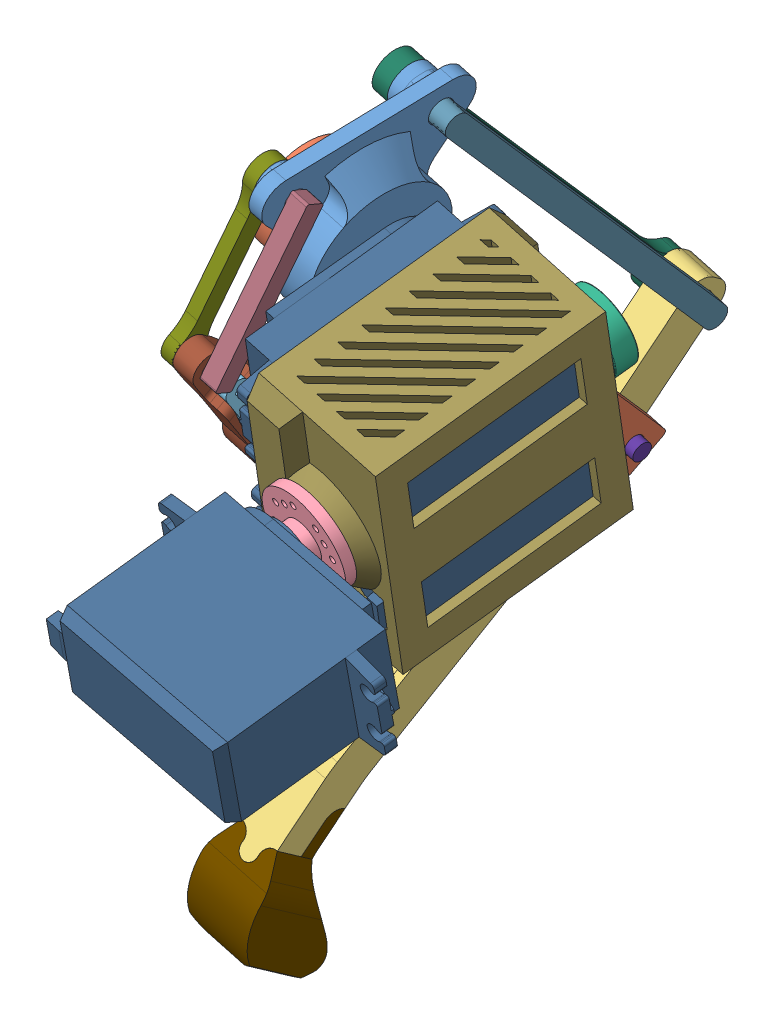
SolidWorks assembly Leg 0, configuration Default. Lengths in mm.
Overall size (103.06 201.69 173.07).
31 component instances, 18 part files, 41 mates.
Components (placement in the parent):
- RearRotatingPiece-1: RearRotatingPiece [Default] at (17.8529 197.1276 29.9823) x (-0.180704 -0.967706 0.175759) z (-0.0444 0.186545 0.981443) size (44.28 13.7 43.21)
- RearUpperLeg-1: RearUpperLeg [Default] at (9.3497 122.3315 -43.4021) x (0.169452 0.64499 -0.745167) z (0.982535 -0.169547 0.076676) size (22 116.4 18)
- RearLowerLeg-1: RearLowerLeg [Default] at (-4.4037 50.9577 33.7008) x (0.037011 0.581891 0.812424) z (-0.982535 0.169547 -0.076676) size (20.21 126 9.59)
- Circle Rudder-1: Circle Rudder [默认] at (18.0109 173.864 63.2452) x (0.470065 -0.866717 -0.166853) z (-0.874709 -0.432175 -0.219336) size (20.8 5.5 20.8)
- Double_Blade_Rudder-1: Double_Blade_Rudder [默认] at (-13.5228 170.7521 41.1436) x (-0.171815 -0.668394 0.723692) z (0.07145 0.724226 0.685851) size (12.2 5.5 38)
- 688ZZ Bearing Assembly-1: 688ZZ Bearing Assembly [Default] at (24.9725 188.558 6.5299) x (0.99278 -0.008575 0.119639) z (-0.117993 -0.24905 0.961276) size (17.99 17.98 5)
  - Outer Ring-1: Outer Ring [Default] at origin size (16 16 5)
  - Inner Ring-1: Inner Ring [Default] x (-0.241565 -0.970385 0) z (0 0 1) size (10.6 10.6 5)
  - Cage-1: Cage [Default] x (0.535517 0.844524 0) z (0 0 1) size (13.01 13.06 2.21)
  - 2mm Ball Bearing-1: 2mm Ball Bearing [Default] at (-5.0671 3.2131 0) x (0.050652 0.835774 0.546732) z (0.977207 -0.154478 0.145614) size (2 2 2)
  - 2mm Ball Bearing-2: 2mm Ball Bearing [Default] at (-5.988 -0.3789 0) x (-0.450278 0.705928 0.546732) z (0.881377 0.449412 0.145614) size (2 2 2)
  - 2mm Ball Bearing-3: 2mm Ball Bearing [Default] at (-4.6217 -3.8262 0) x (-0.779216 0.306441 0.546732) z (0.448891 0.881642 0.145614) size (2 2 2)
  - 2mm Ball Bearing-4: 2mm Ball Bearing [Default] at (-1.49 -5.812 0) x (-0.810521 -0.210096 0.546732) z (-0.155056 0.977115 0.145614) size (2 2 2)
  - 2mm Ball Bearing-5: 2mm Ball Bearing [Default] at (2.2108 -5.5778 0) x (-0.532234 -0.646383 0.546732) z (-0.699777 0.699363 0.145614) size (2 2 2)
  - 2mm Ball Bearing-6: 2mm Ball Bearing [Default] at (5.0671 -3.2131 0) x (-0.050652 -0.835774 0.546732) z (-0.977207 0.154478 0.145614) size (2 2 2)
  - 2mm Ball Bearing-7: 2mm Ball Bearing [Default] at (5.988 0.3789 0) x (0.450278 -0.705928 0.546732) z (-0.881377 -0.449412 0.145614) size (2 2 2)
  - 2mm Ball Bearing-8: 2mm Ball Bearing [Default] at (4.6217 3.8262 0) x (0.779216 -0.306441 0.546732) z (-0.448891 -0.881642 0.145614) size (2 2 2)
  - 2mm Ball Bearing-9: 2mm Ball Bearing [Default] at (1.49 5.812 0) x (0.810521 0.210096 0.546732) z (0.155056 -0.977115 0.145614) size (2 2 2)
  - 2mm Ball Bearing-10: 2mm Ball Bearing [Default] at (-2.2108 5.5778 0) x (0.532234 0.646383 0.546732) z (0.699777 -0.699363 0.145614) size (2 2 2)
- MG996R-3: MG996R [Default] at (23.0553 161.1843 107.4441) x (0.987665 -0.129781 0.087608) z (0.102937 0.959756 0.261291) size (54.5 42.75 20)
- Circle Rudder-2: Circle Rudder [默认] at (-7.0053 201.4171 28.0424) x (-0.185428 -0.85768 0.479585) z (0.015549 0.485427 0.874139) size (20.8 5.5 20.8)
- MG996R-4: MG996R [Default] at (32.1612 165.5985 34.4929) x (0.117993 0.24905 -0.961276) z (0.143886 0.953534 0.264706) size (54.5 42.75 20)
- MG996R-5: MG996R [Default] at (36.0336 191.2606 41.6169) x (-0.117993 -0.24905 0.961276) z (-0.143886 -0.953534 -0.264706) size (54.5 42.75 20)
- Servo Arm Mount-1: Servo Arm Mount [Default] at (-13.6211 170.769 41.1359) x (-0.171815 -0.668394 0.723692) z (-0.982535 0.169547 -0.076676) size (16.2 34.39 10.1)
- RearServoHousing-1: RearServoHousing [Default] at (-3.6223 127.2151 20.1561) x (0.117993 0.24905 -0.961276) z (-0.982535 0.169547 -0.076676) size (61.5 52 29.25)
- RearShortConnectingRod-2: RearShortConnectingRod [Default] at (-49.81 191.4626 52.423) x (0.186018 0.905511 -0.381375) z (-0.982535 0.169547 -0.076676) size (37.08 6.33 13)
- Long Connecting Rod-1: Long Connecting Rod [Default] at (-11.2731 143.0955 -52.7528) x (-0.076888 -0.745152 -0.662447) z (0.982535 -0.169547 0.076676) size (105.4 5 16.7)
- Long Connecting Rod Alt-1: Long Connecting Rod Alt [Default] at (-10.6997 222.7235 12.9444) x (0.076888 0.745152 0.662447) z (-0.169451 -0.644982 0.745174) size (109.5 4 9.1)
- Short Connecting Rod Alt-1: Short Connecting Rod Alt [Default] at (-11.1652 218.4617 43.3941) x (0.186018 0.905511 -0.381375) z (-0.00477 0.388977 0.921235) size (41.18 3 8.1)
- Dowel-1: Dowel [Default] at (-28.4805 128.9748 -39.5446) x (0.103375 0.154723 -0.982535) z (0.982535 -0.169547 0.076676) size (3.9 3.9 20)
- Foot Cap R2-1: Foot Cap R2 [Default] at (-32.8972 55.8746 31.4772) x (0.037011 0.581891 0.812424) z (-0.982535 0.169547 -0.076676) size (26.22 31.5 15)
Mates (geometry in assembly coordinates):
- Concentric12: concentric aligned: cylinder of Circle Rudder-2 through (-4.7454 201.0272 28.2187) axis (-0.982535 0.169547 -0.076676) radius 1.5; cylinder of MG996R-5 through (-1.7978 200.5185 28.4488) axis (-0.982535 0.169547 -0.076676) radius 1.5
- Coincident20: coincident anti-aligned: plane of Circle Rudder-2 through (-4.7454 201.0272 28.2187) normal (0.982535 -0.169547 0.076676); plane of MG996R-5 through (-4.7454 201.0272 28.2187) normal (-0.982535 0.169547 -0.076676)
- Coincident21: coincident anti-aligned: plane of RearUpperLeg-1 through (-7.0053 201.4171 28.0424) normal (0.982535 -0.169547 0.076676); plane of Circle Rudder-2 through (-7.0053 201.4171 28.0424) normal (-0.982535 0.169547 -0.076676)
- Concentric13: concentric anti-aligned: cylinder of RearUpperLeg-1 through (-15.8481 202.9431 27.3523) axis (0.982535 -0.169547 0.076676) radius 1.7; cylinder of Circle Rudder-2 through (-4.7454 201.0272 28.2187) axis (-0.982535 0.169547 -0.076676) radius 1.5
- Concentric14: concentric anti-aligned: cylinder of RearRotatingPiece-1 through (-3.7629 200.8576 28.2954) axis (0.982535 -0.169547 0.076676) radius 4.35; cylinder of Circle Rudder-2 through (-1.6013 200.4846 28.4641) axis (-0.982535 0.169547 -0.076676) radius 4.4
- Coincident22: coincident anti-aligned: plane of RearRotatingPiece-1 through (-1.7978 200.5185 28.4488) normal (0.982535 -0.169547 0.076676); plane of MG996R-5 through (-1.7978 200.5185 28.4488) normal (-0.982535 0.169547 -0.076676)
- Concentric16: concentric aligned: cylinder of Double_Blade_Rudder-1 through (-11.263 170.3621 41.3199) axis (-0.982535 0.169547 -0.076676) radius 1.5; cylinder of MG996R-4 through (-8.1189 169.8196 41.5653) axis (-0.982535 0.169547 -0.076676) radius 1.5
- Coincident24: coincident anti-aligned: plane of Double_Blade_Rudder-1 through (-8.1189 169.8196 41.5653) normal (0.982535 -0.169547 0.076676); plane of MG996R-4 through (-8.1189 169.8196 41.5653) normal (-0.982535 0.169547 -0.076676)
- Concentric23: concentric aligned: cylinder of RearUpperLeg-1 through (-10.7948 125.9229 -38.1645) axis (-0.982535 0.169547 -0.076676) radius 2.1; cylinder of RearLowerLeg-1 through (-15.2163 126.6859 -38.5095) axis (-0.982535 0.169547 -0.076676) radius 2
- Concentric29: concentric aligned: cylinder of Circle Rudder-1 through (17.7395 173.2912 65.4561) axis (0.117993 0.24905 -0.961276) radius 1.5; cylinder of MG996R-3 through (17.3855 172.544 68.34) axis (0.117993 0.24905 -0.961276) radius 1.5
- Coincident34: coincident anti-aligned: plane of Circle Rudder-1 through (17.7395 173.2912 65.4561) normal (-0.117993 -0.24905 0.961276); plane of MG996R-3 through (17.7395 173.2912 65.4561) normal (0.117993 0.24905 -0.961276)
- Concentric32: concentric aligned: cylinder of 688ZZ Bearing Assembly-1/Inner Ring-1 through (24.1754 186.8755 13.0237) axis (-0.117993 -0.24905 0.961276) radius 4; cylinder of RearServoHousing-1 through (25.2674 189.1806 4.1267) axis (-0.117993 -0.24905 0.961276) radius 4
- Coincident40: coincident anti-aligned: plane of Circle Rudder-1 through (18.0109 173.864 63.2452) normal (0.117993 0.24905 -0.961276); plane of RearServoHousing-1 through (103.0236 146.4754 66.5843) normal (-0.117993 -0.24905 0.961276)
- Concentric33: concentric anti-aligned: cylinder of MG996R-5 through (6.9963 194.2046 64.8225) axis (-0.982535 0.169547 -0.076676) radius 1.7678; circle of RearServoHousing-1
- Parallel2: parallel anti-aligned: plane of MG996R-5 through (4.7362 211.9005 22.0569) normal (0.143886 0.953534 0.264706); plane of RearServoHousing-1 through (111.4188 187.5893 49.9189) normal (-0.143886 -0.953534 -0.264706)
- Coincident42: coincident anti-aligned: plane of MG996R-5 through (36.0336 191.2606 41.6169) normal (0.982535 -0.169547 0.076676); plane of RearServoHousing-1 through (32.2269 166.0336 34.6137) normal (-0.982535 0.169547 -0.076676)
- Parallel3: parallel anti-aligned: plane of MG996R-4 through (-3.9149 176.1519 53.8647) normal (0.143886 0.953534 0.264706); plane of RearServoHousing-1 through (107.6777 162.7974 43.0366) normal (-0.143886 -0.953534 -0.264706)
- Concentric34: concentric anti-aligned: cylinder of MG996R-4 through (1.7507 159.4423 55.1723) axis (-0.982535 0.169547 -0.076676) radius 1.7678; circle of RearServoHousing-1
- Coincident45: coincident anti-aligned: plane of MG996R-4 through (32.1612 165.5985 34.4929) normal (0.982535 -0.169547 0.076676); plane of RearServoHousing-1 through (32.2269 166.0336 34.6137) normal (-0.982535 0.169547 -0.076676)
- Coincident46: coincident anti-aligned: plane of 688ZZ Bearing Assembly-1/Inner Ring-1 through (29.6657 186.6877 9.2221) normal (-0.117993 -0.24905 0.961276); plane of RearServoHousing-1 through (24.6775 187.9353 8.9331) normal (0.117993 0.24905 -0.961276)
- Concentric38: concentric aligned: cylinder of Circle Rudder-1 through (17.3619 172.4942 68.5322) axis (0.117993 0.24905 -0.961276) radius 4.4; circle of RearServoHousing-1
- Distance4: distance = 0.5 mm anti-aligned: plane of RearLowerLeg-1 through (-41.74 57.4005 30.7871) normal (-0.982535 0.169547 -0.076676); plane of RearUpperLeg-1 through (-26.7677 117.7763 -34.0864) normal (0.982535 -0.169547 0.076676)
- Concentric39: concentric anti-aligned: cylinder of Double_Blade_Rudder-1 through (-11.263 170.3621 41.3199) axis (-0.982535 0.169547 -0.076676) radius 1.5; cylinder of Servo Arm Mount-1 through (-16.5687 171.2777 40.9059) axis (0.982535 -0.169547 0.076676) radius 1.7
- Concentric40: concentric aligned: cylinder of Double_Blade_Rudder-1 through (-10.7628 175.4317 46.1209) axis (-0.982535 0.169547 -0.076676) radius 0.75; cylinder of Servo Arm Mount-1 through (-13.0227 175.8217 45.9445) axis (-0.982535 0.169547 -0.076676) radius 0.75
- Coincident49: coincident anti-aligned: plane of Double_Blade_Rudder-1 through (-13.5228 170.7521 41.1436) normal (-0.982535 0.169547 -0.076676); plane of Servo Arm Mount-1 through (-13.5228 170.7521 41.1436) normal (0.982535 -0.169547 0.076676)
- Concentric41: concentric aligned: cylinder of RearRotatingPiece-1 through (-9.1019 218.1056 43.5551) axis (0.982535 -0.169547 0.076676) radius 2.2; cylinder of RearShortConnectingRod-2 through (-14.8006 219.089 43.1104) axis (0.982535 -0.169547 0.076676) radius 2
- Concentric42: concentric anti-aligned: cylinder of Servo Arm Mount-1 through (-7.7828 186.393 56.9521) axis (-0.982535 0.169547 -0.076676) radius 1.7; cylinder of RearShortConnectingRod-2 through (-21.047 188.6819 55.917) axis (0.982535 -0.169547 0.076676) radius 1.5
- Coincident50: coincident anti-aligned: plane of RearRotatingPiece-1 through (-5.9956 218.2931 45.8998) normal (0.982535 -0.169547 0.076676); plane of RearShortConnectingRod-2 through (-12.4737 185.0198 55.3367) normal (-0.982535 0.169547 -0.076676)
- Concentric43: concentric aligned: cylinder of RearShortConnectingRod-2 through (-21.047 188.6819 55.917) axis (0.982535 -0.169547 0.076676) radius 1.5; cylinder of Short Connecting Rod Alt-1 through (-20.3593 188.5632 55.9707) axis (0.982535 -0.169547 0.076676) radius 1.55
- Coincident51: coincident anti-aligned: plane of RearRotatingPiece-1 through (-12.704 202.4005 27.5977) normal (-0.982535 0.169547 -0.076676); plane of Short Connecting Rod Alt-1 through (-11.1652 218.4617 43.3941) normal (0.982535 -0.169547 0.076676)
- Concentric44: concentric aligned: cylinder of RearShortConnectingRod-2 through (-14.8006 219.089 43.1104) axis (0.982535 -0.169547 0.076676) radius 2; cylinder of Short Connecting Rod Alt-1 through (-14.1128 218.9703 43.1641) axis (0.982535 -0.169547 0.076676) radius 2.05
- Concentric45: concentric anti-aligned: cylinder of RearRotatingPiece-1 through (-6.0818 221.9266 13.3047) axis (0.982535 -0.169547 0.076676) radius 2.7; cylinder of Long Connecting Rod-1 through (0.9924 220.7059 13.8568) axis (-0.982535 0.169547 -0.076676) radius 2.5
- Concentric46: concentric aligned: cylinder of RearLowerLeg-1 through (-10.6572 146.5708 -52.9596) axis (-0.982535 0.169547 -0.076676) radius 2.6; cylinder of Long Connecting Rod-1 through (-6.7271 145.8926 -52.6529) axis (-0.982535 0.169547 -0.076676) radius 2.5
- Coincident52: coincident anti-aligned: plane of RearLowerLeg-1 through (-32.8972 55.8746 31.4772) normal (0.982535 -0.169547 0.076676); plane of Long Connecting Rod-1 through (-11.2731 143.0955 -52.7528) normal (-0.982535 0.169547 -0.076676)
- Concentric47: concentric anti-aligned: cylinder of Long Connecting Rod-1 through (-6.7271 145.8926 -52.6529) axis (-0.982535 0.169547 -0.076676) radius 2.5; cylinder of Long Connecting Rod Alt-1 through (-22.3494 148.5884 -53.872) axis (0.982535 -0.169547 0.076676) radius 2.55
- Concentric48: concentric anti-aligned: cylinder of Long Connecting Rod-1 through (0.9924 220.7059 13.8568) axis (-0.982535 0.169547 -0.076676) radius 2.5; cylinder of Long Connecting Rod Alt-1 through (-14.6299 223.4017 12.6377) axis (0.982535 -0.169547 0.076676) radius 2.55
- Coincident53: coincident anti-aligned: plane of RearRotatingPiece-1 through (-10.6997 222.7235 12.9444) normal (-0.982535 0.169547 -0.076676); plane of Long Connecting Rod Alt-1 through (-10.6997 222.7235 12.9444) normal (0.982535 -0.169547 0.076676)
- Concentric49: concentric aligned: cylinder of RearUpperLeg-1 through (-10.7948 125.9229 -38.1645) axis (-0.982535 0.169547 -0.076676) radius 2.1; cylinder of Dowel-1 through (-8.8298 125.5838 -38.0111) axis (-0.982535 0.169547 -0.076676) radius 1.95
- Coincident54: coincident aligned: plane of RearUpperLeg-1 through (-27.9867 128.7743 -46.3157) normal (-0.982535 0.169547 -0.076676); plane of Dowel-1 through (-28.4805 128.9748 -39.5446) normal (-0.982535 0.169547 -0.076676)
- Concentric50: concentric aligned: cylinder of RearLowerLeg-1 through (-33.5829 70.8291 14.643) axis (-0.037011 -0.581891 -0.812424) radius 2; cylinder of Foot Cap R2-1 through (-33.5829 70.8291 14.643) axis (-0.037011 -0.581891 -0.812424) radius 2
- Concentric51: concentric anti-aligned: cylinder of RearLowerLeg-1 through (-40.8309 59.2634 23.257) axis (0.982535 -0.169547 0.076676) radius 2; cylinder of Foot Cap R2-1 through (-31.9881 57.7375 23.9471) axis (-0.982535 0.169547 -0.076676) radius 2
